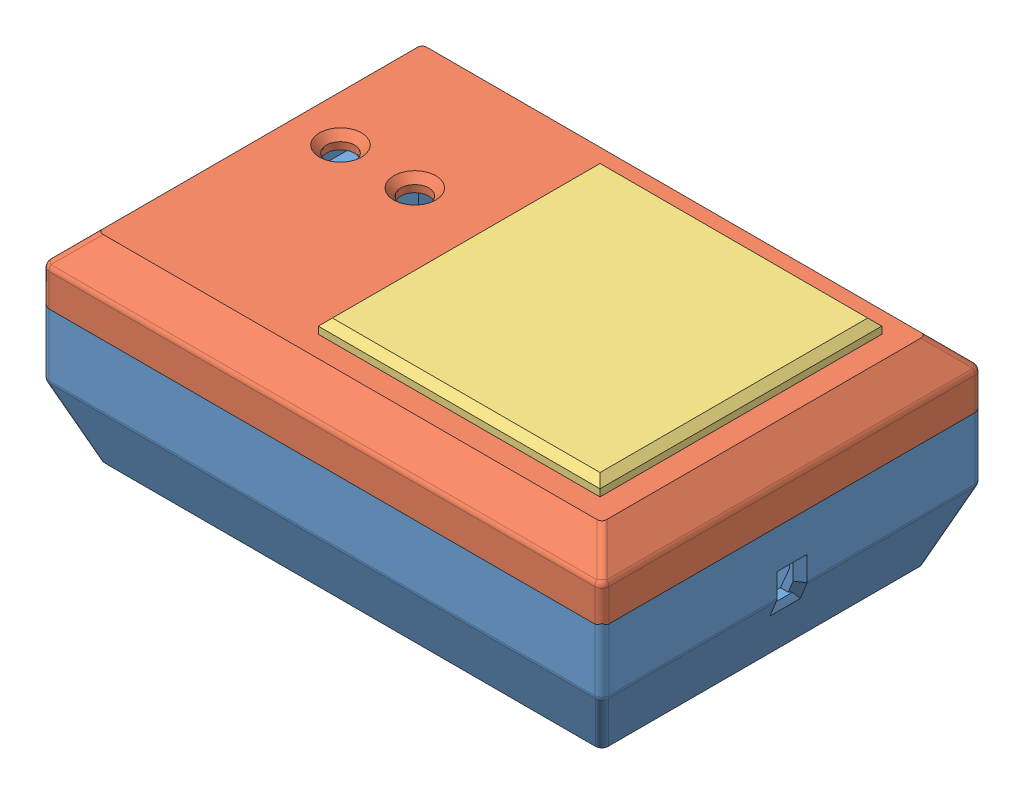
SolidWorks assembly case_mood_v2, configuration Default. Lengths in mm.
Overall size (79.5 30 54).
107 component instances, 26 part files, 15 mates.
Components (placement in the parent):
- Part1^case_mood_v2-1: Part1^case_mood_v2 [Default] x (1 0 0) z (0 1 0) size (79.5 54 20) (virtual)
- mood-mood.step-1: mood-mood.step [Default] at (2.5 1.6 -10) x (1 0 0) z (0 1 0) size (76.01 40 14.44) (hidden)
  - Board_Geoms_e038.step-1: Board_Geoms_e038.step [Default] at origin size (75 40 1.6)
    - Pcb_e038.step-1: Pcb_e038.step [Default] at (-147.1 99.5 0) size (75 40 1.6)
  - Step_Models_e038.step-1: Step_Models_e038.step [Default] at origin size (71.91 38.55 14.44)
    - Top_e038.step-1: Top_e038.step [Default] at origin size (71.91 38.55 7.8)
      - IC2_DRL0006A_ASM_d850ca76bd89.step-1: IC2_DRL0006A_ASM_d850ca76bd89.step [Default] at (-11.65 2.75 0) size (1.6 1.6 0.6)
        - FRAME-DRL0006A.step-1: FRAME-DRL0006A.step [Default] x (0 1 0) z (1 0 0) size (1.2 0.13 1.6)
          - SOLID.step-1: SOLID.step [Default] at origin size (0.2 0.13 0.3)
          - SOLID001.step-1: SOLID001.step [Default] at origin size (0.2 0.13 0.3)
          - SOLID002.step-1: SOLID002.step [Default] at origin size (0.2 0.13 0.3)
          - SOLID003.step-1: SOLID003.step [Default] at origin size (0.2 0.13 0.3)
          - SOLID004.step-1: SOLID004.step [Default] at origin size (0.2 0.13 0.3)
          - SOLID005.step-1: SOLID005.step [Default] at origin size (0.2 0.13 0.3)
        - BODY-SOT.step-1: BODY-SOT.step [Default] at (0 0 0.025) x (0 1 0) z (1 0 0) size (1.6 0.58 1.2)
      - IC6_ASSEMBLY_ace8437915b6.step-1: IC6_ASSEMBLY_ace8437915b6.step [Default] at (-21.4 7.5 0) size (2.1 2 0.6)
        - Body.step-1: Body.step [Default] at origin size (2 2 0.55)
        - ThermalPin.step-1: ThermalPin.step [Default] at (-0.3875 -0.8375 0) size (0.78 1.68 0.07)
        - PinsArrayLR.step-1: PinsArrayLR.step [Default] at origin size (2.1 1.24 0.07)
      - R52_R_0402_1005Metric_0573c14c30cb.step-1: R52_R_0402_1005Metric_0573c14c30cb.step [Default] at (15.2 -25 0) x (-1 0 0) z (0 0 1) size (1 0.5 0.35)
      - R52_R_0402_1005Metric_0573c14c30cb.step-2: R52_R_0402_1005Metric_0573c14c30cb.step [Default] at (30.2 6.8 0) x (-1 0 0) z (0 0 1) size (1 0.5 0.35)
      - R52_R_0402_1005Metric_0573c14c30cb.step-3: R52_R_0402_1005Metric_0573c14c30cb.step [Default] at (15.2 -6.8 0) x (-1 0 0) z (0 0 1) size (1 0.5 0.35)
      - D4_LED_RGB_5050_6_5aed774da48c.step-1: D4_LED_RGB_5050_6_5aed774da48c.step [Default] at (25 5 0) size (5.4 5 1.6)
      - R52_R_0402_1005Metric_0573c14c30cb.step-4: R52_R_0402_1005Metric_0573c14c30cb.step [Default] at (0.2 -23.2 0) x (-1 0 0) z (0 0 1) size (1 0.5 0.35)
      - IC1_ESP32-C3-WROOM-02-H4_28caeafe01dd.step-1: IC1_ESP32-C3-WROOM-02-H4_28caeafe01dd.step [Default] at (-26.65 -20 0.4) x (-1 0 0) z (0 0 1) size (18 20 3.2)
      - R2_R_0603_1608Metric_003f984474a4.step-1: R2_R_0603_1608Metric_003f984474a4.step [Default] at (-8.65 0 0) x (0 -1 0) z (0 0 1) size (1.6 0.8 0.45)
      - C5_C_0805_2012Metric_cb7698a6af10.step-1: C5_C_0805_2012Metric_cb7698a6af10.step [Default] at (-11.65 0.25 0) size (2 1.25 1.25)
      - R52_R_0402_1005Metric_0573c14c30cb.step-5: R52_R_0402_1005Metric_0573c14c30cb.step [Default] at (30.4 -13.2 0) x (-1 0 0) z (0 0 1) size (1 0.5 0.35)
      - D4_LED_RGB_5050_6_5aed774da48c.step-2: D4_LED_RGB_5050_6_5aed774da48c.step [Default] at (-5 5 0) size (5.4 5 1.6)
      - R52_R_0402_1005Metric_0573c14c30cb.step-6: R52_R_0402_1005Metric_0573c14c30cb.step [Default] at (15.2 -5 0) x (-1 0 0) z (0 0 1) size (1 0.5 0.35)
      - D4_LED_RGB_5050_6_5aed774da48c.step-3: D4_LED_RGB_5050_6_5aed774da48c.step [Default] at (-5 -15 0) size (5.4 5 1.6)
      - R52_R_0402_1005Metric_0573c14c30cb.step-7: R52_R_0402_1005Metric_0573c14c30cb.step [Default] at (15.2 3.2 0) x (-1 0 0) z (0 0 1) size (1 0.5 0.35)
      - D4_LED_RGB_5050_6_5aed774da48c.step-4: D4_LED_RGB_5050_6_5aed774da48c.step [Default] at (10 -15 0) size (5.4 5 1.6)
      - R2_R_0603_1608Metric_003f984474a4.step-2: R2_R_0603_1608Metric_003f984474a4.step [Default] at (-38.1 -17.8 0) x (0 1 0) z (0 0 1) size (1.6 0.8 0.45)
      - R52_R_0402_1005Metric_0573c14c30cb.step-8: R52_R_0402_1005Metric_0573c14c30cb.step [Default] at (30.4 -3.2 0) x (-1 0 0) z (0 0 1) size (1 0.5 0.35)
      - J2_12401610E42A_931c68c1d1c5[2].step-1: J2_12401610E42A_931c68c1d1c5[2].step [Default] at (-41 3.8 1.5) x (-1 0 0) z (0 0 1) size (10.51 9.21 4.22)
      - R2_R_0603_1608Metric_003f984474a4.step-3: R2_R_0603_1608Metric_003f984474a4.step [Default] at (-19 1.6 0) x (0 -1 0) z (0 0 1) size (1.6 0.8 0.45)
      - D4_LED_RGB_5050_6_5aed774da48c.step-5: D4_LED_RGB_5050_6_5aed774da48c.step [Default] at (10 -25 0) size (5.4 5 1.6)
      - R52_R_0402_1005Metric_0573c14c30cb.step-9: R52_R_0402_1005Metric_0573c14c30cb.step [Default] at (30.4 -16.8 0) x (-1 0 0) z (0 0 1) size (1 0.5 0.35)
      - R2_R_0603_1608Metric_003f984474a4.step-4: R2_R_0603_1608Metric_003f984474a4.step [Default] at (-4.65 0.75 0) x (-1 0 0) z (0 0 1) size (1.6 0.8 0.45)
      - R52_R_0402_1005Metric_0573c14c30cb.step-10: R52_R_0402_1005Metric_0573c14c30cb.step [Default] at (15.2025 5 0) x (-1 0 0) z (0 0 1) size (1 0.5 0.35)
      - R2_R_0603_1608Metric_003f984474a4.step-5: R2_R_0603_1608Metric_003f984474a4.step [Default] at (4.5875 -7.2687 0) size (1.6 0.8 0.45)
      - D2_LED_0805_2012Metric_59915ddbd9d1.step-1: D2_LED_0805_2012Metric_59915ddbd9d1.step [Default] at (-21 1.6 0) x (0 -1 0) z (0 0 1) size (2 1.25 1.1)
      - D4_LED_RGB_5050_6_5aed774da48c.step-6: D4_LED_RGB_5050_6_5aed774da48c.step [Default] at (-5 -25 0) size (5.4 5 1.6)
      - R52_R_0402_1005Metric_0573c14c30cb.step-11: R52_R_0402_1005Metric_0573c14c30cb.step [Default] at (0.2 -25 0) x (-1 0 0) z (0 0 1) size (1 0.5 0.35)
      - R52_R_0402_1005Metric_0573c14c30cb.step-12: R52_R_0402_1005Metric_0573c14c30cb.step [Default] at (0.2 3.2 0) x (-1 0 0) z (0 0 1) size (1 0.5 0.35)
      - R52_R_0402_1005Metric_0573c14c30cb.step-13: R52_R_0402_1005Metric_0573c14c30cb.step [Default] at (15.2 -23.2 0) x (-1 0 0) z (0 0 1) size (1 0.5 0.35)
      - R2_R_0603_1608Metric_003f984474a4.step-6: R2_R_0603_1608Metric_003f984474a4.step [Default] at (-14.3 -20.8 0) x (-1 0 0) z (0 0 1) size (1.6 0.8 0.45)
      - R52_R_0402_1005Metric_0573c14c30cb.step-14: R52_R_0402_1005Metric_0573c14c30cb.step [Default] at (30.4 -25 0) x (-1 0 0) z (0 0 1) size (1 0.5 0.35)
      - C11_C_0603_1608Metric_8816bd15a2e3.step-1: C11_C_0603_1608Metric_8816bd15a2e3.step [Default] at (-18.65 7.75 0) x (0 1 0) z (0 0 1) size (1.6 0.8 0.8)
      - D4_LED_RGB_5050_6_5aed774da48c.step-7: D4_LED_RGB_5050_6_5aed774da48c.step [Default] at (25 -25 0) size (5.4 5 1.6)
      - R52_R_0402_1005Metric_0573c14c30cb.step-15: R52_R_0402_1005Metric_0573c14c30cb.step [Default] at (0.2 -3.2 0) x (-1 0 0) z (0 0 1) size (1 0.5 0.35)
      - R2_R_0603_1608Metric_003f984474a4.step-7: R2_R_0603_1608Metric_003f984474a4.step [Default] at (-27.2 0.8 0) x (0 1 0) z (0 0 1) size (1.6 0.8 0.45)
      - C11_C_0603_1608Metric_8816bd15a2e3.step-2: C11_C_0603_1608Metric_8816bd15a2e3.step [Default] at (-11.65 -4 0) size (1.6 0.8 0.8)
      - R52_R_0402_1005Metric_0573c14c30cb.step-16: R52_R_0402_1005Metric_0573c14c30cb.step [Default] at (30.4 -15 0) x (-1 0 0) z (0 0 1) size (1 0.5 0.35)
      - R52_R_0402_1005Metric_0573c14c30cb.step-17: R52_R_0402_1005Metric_0573c14c30cb.step [Default] at (0.2 5 0) x (-1 0 0) z (0 0 1) size (1 0.5 0.35)
      - C11_C_0603_1608Metric_8816bd15a2e3.step-3: C11_C_0603_1608Metric_8816bd15a2e3.step [Default] at (-7.15 0 0) x (0 1 0) z (0 0 1) size (1.6 0.8 0.8)
      - R52_R_0402_1005Metric_0573c14c30cb.step-18: R52_R_0402_1005Metric_0573c14c30cb.step [Default] at (0.2 -6.8 0) x (-1 0 0) z (0 0 1) size (1 0.5 0.35)
      - R2_R_0603_1608Metric_003f984474a4.step-8: R2_R_0603_1608Metric_003f984474a4.step [Default] at (-14.3 -14.4 0) x (-1 0 0) z (0 0 1) size (1.6 0.8 0.45)
      - D4_LED_RGB_5050_6_5aed774da48c.step-8: D4_LED_RGB_5050_6_5aed774da48c.step [Default] at (25 -15 0) size (5.4 5 1.6)
      - R52_R_0402_1005Metric_0573c14c30cb.step-19: R52_R_0402_1005Metric_0573c14c30cb.step [Default] at (30.2 5 0) x (-1 0 0) z (0 0 1) size (1 0.5 0.35)
      - R2_R_0603_1608Metric_003f984474a4.step-9: R2_R_0603_1608Metric_003f984474a4.step [Default] at (4.5875 -17.2063 0) size (1.6 0.8 0.45)
      - D4_LED_RGB_5050_6_5aed774da48c.step-9: D4_LED_RGB_5050_6_5aed774da48c.step [Default] at (10 -5 0) size (5.4 5 1.6)
      - R2_R_0603_1608Metric_003f984474a4.step-10: R2_R_0603_1608Metric_003f984474a4.step [Default] at (-14.3 -17.6 0) size (1.6 0.8 0.45)
      - R2_R_0603_1608Metric_003f984474a4.step-11: R2_R_0603_1608Metric_003f984474a4.step [Default] at (-25.2 1.6 0) x (0 -1 0) z (0 0 1) size (1.6 0.8 0.45)
      - R52_R_0402_1005Metric_0573c14c30cb.step-20: R52_R_0402_1005Metric_0573c14c30cb.step [Default] at (30.4 -6.8 0) x (-1 0 0) z (0 0 1) size (1 0.5 0.35)
      - R2_R_0603_1608Metric_003f984474a4.step-12: R2_R_0603_1608Metric_003f984474a4.step [Default] at (-38.1 -14.4 0) x (0 1 0) z (0 0 1) size (1.6 0.8 0.45)
      - R52_R_0402_1005Metric_0573c14c30cb.step-21: R52_R_0402_1005Metric_0573c14c30cb.step [Default] at (15.2 6.8 0) x (-1 0 0) z (0 0 1) size (1 0.5 0.35)
      - R52_R_0402_1005Metric_0573c14c30cb.step-22: R52_R_0402_1005Metric_0573c14c30cb.step [Default] at (15.2025 -3.2 0) x (-1 0 0) z (0 0 1) size (1 0.5 0.35)
      - R52_R_0402_1005Metric_0573c14c30cb.step-23: R52_R_0402_1005Metric_0573c14c30cb.step [Default] at (30.2 3.2 0) x (-1 0 0) z (0 0 1) size (1 0.5 0.35)
      - Q2_SOT_23_dd72da5cd8d7.step-1: Q2_SOT_23_dd72da5cd8d7.step [Default] at (4.55 -24.1188 0) x (0 1 0) z (0 0 1) size (2.5 3 1.2)
      - R52_R_0402_1005Metric_0573c14c30cb.step-24: R52_R_0402_1005Metric_0573c14c30cb.step [Default] at (30.4 -26.8 0) x (-1 0 0) z (0 0 1) size (1 0.5 0.35)
      - C11_C_0603_1608Metric_8816bd15a2e3.step-4: C11_C_0603_1608Metric_8816bd15a2e3.step [Default] at (-11.7 -19.9 0) x (0 1 0) z (0 0 1) size (1.6 0.8 0.8)
      - R2_R_0603_1608Metric_003f984474a4.step-13: R2_R_0603_1608Metric_003f984474a4.step [Default] at (-38.1 -21.3 0) x (0 1 0) z (0 0 1) size (1.6 0.8 0.45)
      - C5_C_0805_2012Metric_cb7698a6af10.step-2: C5_C_0805_2012Metric_cb7698a6af10.step [Default] at (-10.65 7 0) size (2 1.25 1.25)
      - SW2_SW_PUSH_6mm_h4.3mm_68b5b15dd36c.step-1: SW2_SW_PUSH_6mm_h4.3mm_68b5b15dd36c.step [Default] at (-18 -7.4 0) x (-1 0 0) z (0 0 1) size (7.17 6 7.8)
      - R52_R_0402_1005Metric_0573c14c30cb.step-25: R52_R_0402_1005Metric_0573c14c30cb.step [Default] at (15.2 -13.2 0) x (-1 0 0) z (0 0 1) size (1 0.5 0.35)
      - R52_R_0402_1005Metric_0573c14c30cb.step-26: R52_R_0402_1005Metric_0573c14c30cb.step [Default] at (15.2 -26.8 0) x (-1 0 0) z (0 0 1) size (1 0.5 0.35)
      - R2_R_0603_1608Metric_003f984474a4.step-14: R2_R_0603_1608Metric_003f984474a4.step [Default] at (-21.4 5.25 0) size (1.6 0.8 0.45)
      - C11_C_0603_1608Metric_8816bd15a2e3.step-5: C11_C_0603_1608Metric_8816bd15a2e3.step [Default] at (-14.3 -22.5 0) size (1.6 0.8 0.8)
      - D4_LED_RGB_5050_6_5aed774da48c.step-10: D4_LED_RGB_5050_6_5aed774da48c.step [Default] at (25 -5 0) size (5.4 5 1.6)
      - SW2_SW_PUSH_6mm_h4.3mm_68b5b15dd36c.step-2: SW2_SW_PUSH_6mm_h4.3mm_68b5b15dd36c.step [Default] at (-34.85 -2.9 0) size (7.17 6 7.8)
      - R52_R_0402_1005Metric_0573c14c30cb.step-27: R52_R_0402_1005Metric_0573c14c30cb.step [Default] at (0.2 -5 0) x (-1 0 0) z (0 0 1) size (1 0.5 0.35)
      - R2_R_0603_1608Metric_003f984474a4.step-15: R2_R_0603_1608Metric_003f984474a4.step [Default] at (-29 0.8 0) x (0 1 0) z (0 0 1) size (1.6 0.8 0.45)
      - C5_C_0805_2012Metric_cb7698a6af10.step-3: C5_C_0805_2012Metric_cb7698a6af10.step [Default] at (-11.65 -2 0) size (2 1.25 1.25)
      - D4_LED_RGB_5050_6_5aed774da48c.step-11: D4_LED_RGB_5050_6_5aed774da48c.step [Default] at (10 5 0) size (5.4 5 1.6)
      - R52_R_0402_1005Metric_0573c14c30cb.step-28: R52_R_0402_1005Metric_0573c14c30cb.step [Default] at (15.2 -16.8 0) x (-1 0 0) z (0 0 1) size (1 0.5 0.35)
      - L1_L_Wuerth_MAPI_4020_5ef69c3bf382.step-1: L1_L_Wuerth_MAPI_4020_5ef69c3bf382.step [Default] at (-15.65 1.75 0) x (0 1 0) z (0 0 1) size (3 4 2)
      - R2_R_0603_1608Metric_003f984474a4.step-16: R2_R_0603_1608Metric_003f984474a4.step [Default] at (-14.3 -19.2 0) x (-1 0 0) z (0 0 1) size (1.6 0.8 0.45)
      - R52_R_0402_1005Metric_0573c14c30cb.step-29: R52_R_0402_1005Metric_0573c14c30cb.step [Default] at (30.4 -23.2 0) x (-1 0 0) z (0 0 1) size (1 0.5 0.35)
      - Q2_SOT_23_dd72da5cd8d7.step-2: Q2_SOT_23_dd72da5cd8d7.step [Default] at (4.55 -4.0688 0) x (0 1 0) z (0 0 1) size (2.5 3 1.2)
      - D4_LED_RGB_5050_6_5aed774da48c.step-12: D4_LED_RGB_5050_6_5aed774da48c.step [Default] at (-5 -5 0) size (5.4 5 1.6)
      - C11_C_0603_1608Metric_8816bd15a2e3.step-6: C11_C_0603_1608Metric_8816bd15a2e3.step [Default] at (-10.65 5 0) size (1.6 0.8 0.8)
      - R52_R_0402_1005Metric_0573c14c30cb.step-30: R52_R_0402_1005Metric_0573c14c30cb.step [Default] at (0.2 -13.2 0) x (-1 0 0) z (0 0 1) size (1 0.5 0.35)
      - R52_R_0402_1005Metric_0573c14c30cb.step-31: R52_R_0402_1005Metric_0573c14c30cb.step [Default] at (0.2 -15 0) x (-1 0 0) z (0 0 1) size (1 0.5 0.35)
      - R52_R_0402_1005Metric_0573c14c30cb.step-32: R52_R_0402_1005Metric_0573c14c30cb.step [Default] at (0.2 -26.8 0) x (-1 0 0) z (0 0 1) size (1 0.5 0.35)
      - D2_LED_0805_2012Metric_59915ddbd9d1.step-2: D2_LED_0805_2012Metric_59915ddbd9d1.step [Default] at (-23.2 1.6 0) x (0 -1 0) z (0 0 1) size (2 1.25 1.1)
      - R52_R_0402_1005Metric_0573c14c30cb.step-33: R52_R_0402_1005Metric_0573c14c30cb.step [Default] at (0.2 6.8 0) x (-1 0 0) z (0 0 1) size (1 0.5 0.35)
      - R2_R_0603_1608Metric_003f984474a4.step-17: R2_R_0603_1608Metric_003f984474a4.step [Default] at (4.55 -27.0188 0) size (1.6 0.8 0.45)
      - R52_R_0402_1005Metric_0573c14c30cb.step-34: R52_R_0402_1005Metric_0573c14c30cb.step [Default] at (0.2 -16.8 0) x (-1 0 0) z (0 0 1) size (1 0.5 0.35)
      - Q2_SOT_23_dd72da5cd8d7.step-3: Q2_SOT_23_dd72da5cd8d7.step [Default] at (4.55 -14.0687 0) x (0 1 0) z (0 0 1) size (2.5 3 1.2)
      - R52_R_0402_1005Metric_0573c14c30cb.step-35: R52_R_0402_1005Metric_0573c14c30cb.step [Default] at (15.2 -15 0) x (-1 0 0) z (0 0 1) size (1 0.5 0.35)
      - R52_R_0402_1005Metric_0573c14c30cb.step-36: R52_R_0402_1005Metric_0573c14c30cb.step [Default] at (30.4 -5 0) x (-1 0 0) z (0 0 1) size (1 0.5 0.35)
    - Bot_e038.step-1: Bot_e038.step [Default] at origin size (5.08 7.62 11.54)
      - J1_PinHeader_2x03_P254mm_Vertical_e1aae7fb38ca.step-1: J1_PinHeader_2x03_P254mm_Vertical_e1aae7fb38ca.step [Default] at (-24.275 -19.525 -1.6) x (1 0 0) z (0 0 -1) size (5.08 7.62 11.54) (hidden)
- Part25^case_mood_v2-1: Part25^case_mood_v2 [Default] x (1 0 0) z (0 1 0) size (79.5 54 9) (virtual)
- Part26^case_mood_v2-1: Part26^case_mood_v2 [Default] at (0 8 0) x (1 0 0) z (0 1 0) size (40 40 8.4) (virtual)
Mates (geometry in assembly coordinates):
- InPlace1: in place: plane of ? through (0 0 0) normal (0 1 0); moOrthogonalPlaneRef_w of ? through (0 0 0) normal (0 0 -1); plane of ? through (0 0 0) normal (1 0 0); unknown of ?
- Coincident1: coincident aligned: 
- Coincident2: coincident aligned: plane of Part1^case_mood_v2-1 through (0 0 0) normal (0 0 -1)
- Coincident3: coincident anti-aligned: plane of Part1^case_mood_v2-1 through (0 0 0) normal (1 0 0)
- Width1: width anti-aligned: plane of mood-mood.step-1/Board_Geoms_e038.step-1/Pcb_e038.step-1 through (37.5 1.6 18) normal (1 0 0); plane of Part1^case_mood_v2-1 through (-37.5 1.6 -18) normal (-1 0 0); plane of mood-mood.step-1/Board_Geoms_e038.step-1/Pcb_e038.step-1 through (-39.75 -20 0) normal (-1 0 0); plane of Part1^case_mood_v2-1 through (39.75 -20 0) normal (1 0 0)
- Coincident5: coincident anti-aligned: plane of Part1^case_mood_v2-1 through (0 0 0) normal (0 1 0); plane of mood-mood.step-1/Board_Geoms_e038.step-1/Pcb_e038.step-1 through (0.8484 0 -0.8827) normal (0 -1 0)
- Width2: width anti-aligned: plane of mood-mood.step-1/Board_Geoms_e038.step-1/Pcb_e038.step-1 through (35.5 1.6 -20) normal (0 0 -1); plane of Part1^case_mood_v2-1 through (-7.5 1.6 20) normal (0 0 1); plane of mood-mood.step-1/Board_Geoms_e038.step-1/Pcb_e038.step-1 through (0 -20 27) normal (0 0 1); plane of Part1^case_mood_v2-1 through (0 -20 -27) normal (0 0 -1)
- InPlace2: in place: plane of ? through (0 0 0) normal (0 1 0); plane of ? through (0 0 0) normal (0 1 0); plane of ? through (0 0 0) normal (0 1 0); plane of ? through (0 0 0) normal (0 0 -1); plane of ? through (0 0 0) normal (0 1 0); plane of ? through (0 0 0) normal (1 0 0); plane of ? through (0 0 0) normal (0 1 0); unknown of ?
- Coincident6: coincident aligned: plane of ?; plane of ?
- Coincident7: coincident aligned: moOrthogonalPlaneRef_w of Part1^case_mood_v2-1 through (0 0 0) normal (0 0 -1); plane of Part25^case_mood_v2-1 through (0 0 0) normal (0 0 -1)
- Coincident8: coincident anti-aligned: moOrthogonalPlaneRef_w of Part1^case_mood_v2-1 through (0 0 0) normal (-1 0 0); plane of Part25^case_mood_v2-1 through (0 0 0) normal (1 0 0)
- InPlace3: in place: plane of ? through (0 8 0) normal (0 1 0); plane of Part26^case_mood_v2-1 through (0 8 0) normal (0 1 0); plane of ? through (0 8 0) normal (0 1 0); plane of Part26^case_mood_v2-1 through (0 8 0) normal (0 0 -1); plane of ? through (0 8 0) normal (0 1 0); plane of Part26^case_mood_v2-1 through (0 8 0) normal (1 0 0); plane of ? through (0 8 0) normal (0 1 0); unknown of Part26^case_mood_v2-1
- Coincident9: coincident aligned: plane of ?; plane of ?
- Coincident10: coincident aligned: moOrthogonalPlaneRef_w of Part25^case_mood_v2-1 through (0 8 0) normal (0 0 -1); plane of Part26^case_mood_v2-1 through (0 8 0) normal (0 0 -1)
- Coincident11: coincident anti-aligned: moOrthogonalPlaneRef_w of Part25^case_mood_v2-1 through (0 8 0) normal (-1 0 0); plane of Part26^case_mood_v2-1 through (0 8 0) normal (1 0 0)
